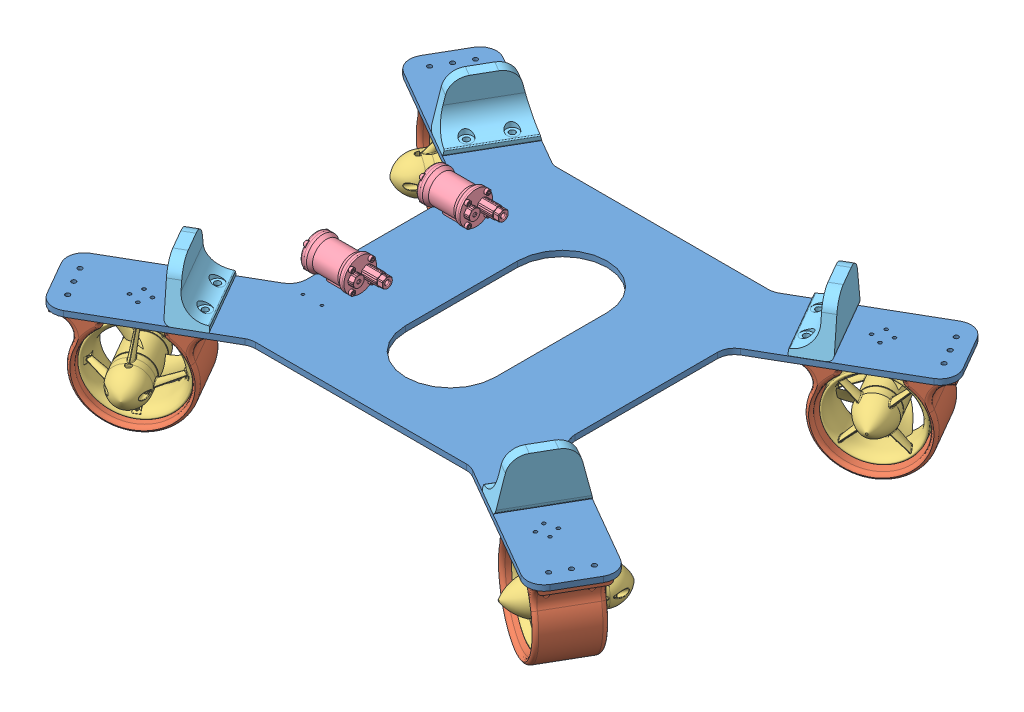
SolidWorks assembly CR-SA-003-HorizontalMotorsAndMount, configuration Default. Lengths in mm.
Overall size (620.81 551.29 537.72).
19 component instances, 5 part files, 40 mates.
Components (placement in the parent):
- CR-P-0008-MotorMount-1: CR-P-0008-MotorMount [Default] at (-219.9502 -31.4468 156.8428) x (0 0 -1) z (1 0 0) size (503.61 6.35 620.81)
- CR-SA-HorizontalThrusterAndMount-1: CR-SA-HorizontalThrusterAndMount [Default] at (-314.8315 -31.4468 365.9541) x (0.866025 0 -0.5) z (-0.5 0 -0.866025) size (139.7 110.81 112.68)
  - CR-P-0005b-Frame-MotorMount Horizontal-1: CR-P-0005b-Frame-MotorMount Horizontal [Default] at (0 55.5625 -5.427) x (0 -1 0) z (0 0 1) size (110.81 139.7 64.82)
  - CR-P-0003-T200-THRUSTER-R1-1: CR-P-0003-T200-THRUSTER-R1 [Default] at (0 55.5625 26.323) x (1 0 0) z (0 0 -1) size (96.71 97.53 112.68)
- CR-SA-HorizontalThrusterAndMount-2: CR-SA-HorizontalThrusterAndMount [Default] at (-341.1545 -31.4468 -6.6757) x (0.866025 0 0.5) z (0.5 0 -0.866025) size (139.7 110.81 112.68)
  - CR-P-0005b-Frame-MotorMount Horizontal-1: CR-P-0005b-Frame-MotorMount Horizontal [Default] at (0 55.5625 -5.427) x (0 -1 0) z (0 0 1) size (110.81 139.7 64.82)
  - CR-P-0003-T200-THRUSTER-R1-1: CR-P-0003-T200-THRUSTER-R1 [Default] at (0 55.5625 26.323) x (1 0 0) z (0 0 -1) size (96.71 97.53 112.68)
- CR-SA-HorizontalThrusterAndMount-3: CR-SA-HorizontalThrusterAndMount [Default] at (124.6163 -31.4468 -52.2686) x (-0.866025 0 0.5) z (0.5 0 0.866025) size (139.7 110.81 112.68)
  - CR-P-0005b-Frame-MotorMount Horizontal-1: CR-P-0005b-Frame-MotorMount Horizontal [Default] at (0 55.5625 -5.427) x (0 -1 0) z (0 0 1) size (110.81 139.7 64.82)
  - CR-P-0003-T200-THRUSTER-R1-1: CR-P-0003-T200-THRUSTER-R1 [Default] at (0 55.5625 26.323) x (1 0 0) z (0 0 -1) size (96.71 97.53 112.68)
- CR-SA-HorizontalThrusterAndMount-4: CR-SA-HorizontalThrusterAndMount [Default] at (150.9393 -31.4468 320.3613) x (-0.866025 0 -0.5) z (-0.5 0 0.866025) size (139.7 110.81 112.68)
  - CR-P-0005b-Frame-MotorMount Horizontal-1: CR-P-0005b-Frame-MotorMount Horizontal [Default] at (0 55.5625 -5.427) x (0 -1 0) z (0 0 1) size (110.81 139.7 64.82)
  - CR-P-0003-T200-THRUSTER-R1-1: CR-P-0003-T200-THRUSTER-R1 [Default] at (0 55.5625 26.323) x (1 0 0) z (0 0 -1) size (96.71 97.53 112.68)
- LUMEN-ASM-R3-PUBLIC-1: LUMEN-ASM-R3-PUBLIC [Default] at (-203.5576 -25.0968 -167.9027) x (0 1 0) z (1 0 0) size (38.48 37 78.39)
- LUMEN-ASM-R3-PUBLIC-4: LUMEN-ASM-R3-PUBLIC [Default] at (-203.5576 -25.0968 -299.4807) x (0 1 0) z (1 0 0) size (38.48 37 78.39)
- CR-P-RestingFeet-1: CR-P-RestingFeet [Default] at (-303.4208 3.4782 -15.1387) x (-0.5 0 0.866025) z (0 1 0) size (82.55 38.1 57.15)
- CR-P-RestingFeet-3: CR-P-RestingFeet [Default] at (113.0786 3.4782 -15.3587) x (-0.5 0 -0.866025) z (0 1 0) size (82.55 38.1 57.15)
- CR-P-RestingFeet-4: CR-P-RestingFeet [Default] at (-303.2938 3.4782 329.0442) x (0.5 0 0.866025) z (0 1 0) size (82.55 38.1 57.15)
- CR-P-RestingFeet-5: CR-P-RestingFeet [Default] at (113.2056 3.4782 328.8243) x (0.5 0 -0.866025) z (0 1 0) size (82.55 38.1 57.15)
Mates (geometry in assembly coordinates):
- Coincident2: coincident anti-aligned: plane of CR-P-0006-VectorizedMotorPlate-2 through (-82.6086 0 202.1216) normal (0 -1 0); plane of CR-P-0005b-Frame-MotorMount Horizontal-1 through (-332.933 -31.4468 4.4842) normal (0 1 0)
- Tangent1: tangent anti-aligned: plane of CR-P-0006-VectorizedMotorPlate-2 through (-312.1112 6.35 238.0427) normal (-0.707107 0 0.707107); cylinder of CR-P-0005b-Frame-MotorMount Horizontal-1 through (-389.1249 -26.674 398.9031) axis (0.707107 0 0.707107) radius 33.02
- Coincident6: coincident anti-aligned: plane of CR-P-0005b-Frame-MotorMount Horizontal-1 through (-332.933 -37.7968 4.4842) normal (0 -1 0); plane of CR-P-0003-T200-THRUSTER-R1-1 through (-372.3007 -37.7968 335.9963) normal (0 1 0)
- Coincident7: coincident anti-aligned: plane of CR-P-0006-VectorizedMotorPlate-2 through (-82.6086 0 202.1216) normal (0 -1 0); plane of CR-P-0005b-Frame-MotorMount Horizontal-2 through (-375.955 -31.4468 11.89) normal (0 1 0)
- Tangent3: tangent anti-aligned: plane of CR-P-0006-VectorizedMotorPlate-2 through (146.894 6.35 238.0427) normal (0.707107 0 0.707107); cylinder of CR-P-0005b-Frame-MotorMount Horizontal-2 through (-330.4009 -26.674 57.4441) axis (-0.707107 0 0.707107) radius 33.02
- Coincident9: coincident anti-aligned: plane of CR-P-0003-T200-THRUSTER-R1-2 through (-353.3308 -37.7968 -12.5208) normal (0 1 0); plane of CR-P-0005b-Frame-MotorMount Horizontal-2 through (-375.955 -37.7968 11.89) normal (0 -1 0)
- Coincident10: coincident anti-aligned: plane of CR-P-0005b-Frame-MotorMount Horizontal-2 through (-375.955 -31.4468 11.89) normal (0 1 0); plane of CR-P-0008-MotorMount-1 through (-219.9502 -31.4468 156.8428) normal (0 -1 0)
- Coincident13: coincident anti-aligned: plane of CR-P-0005b-Frame-MotorMount Horizontal-1 through (-332.933 -31.4468 4.4842) normal (0 1 0); plane of CR-P-0008-MotorMount-1 through (-219.9502 -31.4468 156.8428) normal (0 -1 0)
- Coincident14: coincident anti-aligned: plane of CR-P-0008-MotorMount-1 through (-219.9502 -31.4468 156.8428) normal (0 -1 0); plane of CR-SA-HorizontalThrusterAndMount-1/CR-P-0005b-Frame-MotorMount Horizontal-1 through (-343.868 -31.4468 315.6614) normal (0 1 0)
- Coincident15: coincident anti-aligned: plane of CR-P-0008-MotorMount-1 through (-219.9502 -31.4468 156.8428) normal (0 -1 0); plane of CR-SA-HorizontalThrusterAndMount-2/CR-P-0005b-Frame-MotorMount Horizontal-1 through (-312.118 -31.4468 -56.9684) normal (0 1 0)
- Angle1: planar angle = 2.094395 rad anti-aligned: plane of CR-SA-HorizontalThrusterAndMount-1/CR-P-0005b-Frame-MotorMount Horizontal-1 through (-343.868 -87.0093 315.6614) normal (-0.5 0 -0.866025); plane of CR-P-0008-MotorMount-1 through (-247.5076 -25.0968 248.8825) normal (-1 0 0)
- Angle2: planar angle = 2.094395 rad anti-aligned: plane of CR-P-0008-MotorMount-1 through (-247.5076 -25.0968 248.8825) normal (-1 0 0); plane of CR-SA-HorizontalThrusterAndMount-2/CR-P-0005b-Frame-MotorMount Horizontal-1 through (-343.868 -87.0093 -1.9758) normal (-0.5 0 0.866025)
- Coincident18: coincident anti-aligned: plane of CR-P-0008-MotorMount-1 through (-219.9502 -31.4468 156.8428) normal (0 -1 0); plane of CR-SA-HorizontalThrusterAndMount-3/CR-P-0005b-Frame-MotorMount Horizontal-1 through (153.6528 -31.4468 -1.9758) normal (0 1 0)
- Angle3: planar angle = 2.094395 rad anti-aligned: plane of CR-SA-HorizontalThrusterAndMount-3/CR-P-0005b-Frame-MotorMount Horizontal-1 through (153.6528 -87.0093 -1.9758) normal (0.5 0 0.866025); plane of CR-P-0008-MotorMount-1 through (57.2924 -25.0968 248.8825) normal (1 0 0)
- Coincident20: coincident anti-aligned: plane of CR-P-0008-MotorMount-1 through (-219.9502 -31.4468 156.8428) normal (0 -1 0); plane of CR-SA-HorizontalThrusterAndMount-4/CR-P-0005b-Frame-MotorMount Horizontal-1 through (121.9028 -31.4468 370.654) normal (0 1 0)
- Angle4: planar angle = 2.094395 rad anti-aligned: plane of CR-SA-HorizontalThrusterAndMount-4/CR-P-0005b-Frame-MotorMount Horizontal-1 through (153.6528 -87.0093 315.6614) normal (0.5 0 -0.866025); plane of CR-P-0008-MotorMount-1 through (57.2924 -25.0968 248.8825) normal (1 0 0)
- Coincident22: coincident anti-aligned: plane of CR-P-0008-MotorMount-1 through (-219.9502 -31.4468 156.8428) normal (0 -1 0); plane of CR-P-0005b-Frame-MotorMount Horizontal-1 through (-332.933 -31.4468 4.4842) normal (0 1 0)
- Distance2: distance = 3.81 mm aligned: plane of CR-P-0005b-Frame-MotorMount Horizontal-1 through (-393.4249 -87.0093 -30.4408) normal (-0.866025 0 -0.5); plane of CR-P-0008-MotorMount-1 through (-412.4854 -25.0968 -30.447) normal (-0.866025 0 -0.5)
- Distance3: distance = 9.525 mm aligned: plane of CR-P-0005b-Frame-MotorMount Horizontal-1 through (-301.183 -87.0093 -50.5085) normal (0.5 0 -0.866025); plane of CR-P-0008-MotorMount-1 through (-371.2104 -25.0968 -101.9373) normal (0.5 0 -0.866025)
- Coincident23: coincident anti-aligned: plane of CR-P-0008-MotorMount-1 through (-219.9502 -25.0968 156.8428) normal (0 1 0); plane of LUMEN-ASM-R3-PUBLIC-1 through (-203.5576 -25.0968 222.6318) normal (0 -1 0)
- Parallel1: parallel anti-aligned: line of CR-P-0008-MotorMount-1 through (-214.8458 -25.0968 328.2928) axis (1 0 0); cylinder of LUMEN-ASM-R3-PUBLIC-1 through (-203.5576 -5.1118 222.6318) axis (-1 0 0) radius 15.985
- Coincident25: coincident anti-aligned: plane of CR-P-0008-MotorMount-1 through (-219.9502 -25.0968 156.8428) normal (0 1 0); plane of LUMEN-ASM-R3-PUBLIC-3 through (-203.5576 -25.0968 205.6138) normal (0 -1 0)
- Concentric5: concentric anti-aligned: cylinder of CR-P-0008-MotorMount-1 through (-234.8076 -31.4468 222.6318) axis (0 1 0) radius 1.524; cylinder of LUMEN-ASM-R3-PUBLIC-3 through (-234.8076 -25.0968 205.6138) axis (0 -1 0) radius 1.25
- Parallel3: parallel aligned: cylinder of LUMEN-ASM-R3-PUBLIC-1 through (-203.5576 -5.1118 222.6318) axis (-1 0 0) radius 15.985; cylinder of LUMEN-ASM-R3-PUBLIC-3 through (-203.5576 -5.1118 205.6138) axis (-1 0 0) radius 15.985
- Coincident26: coincident anti-aligned: plane of CR-P-0008-MotorMount-1 through (-219.9502 -25.0968 156.8428) normal (0 1 0); plane of LUMEN-ASM-R3-PUBLIC-4 through (-203.5576 -25.0968 91.0538) normal (0 -1 0)
- Parallel5: parallel aligned: cylinder of LUMEN-ASM-R3-PUBLIC-3 through (-203.5576 -5.1118 205.6138) axis (-1 0 0) radius 15.985; cylinder of LUMEN-ASM-R3-PUBLIC-4 through (-203.5576 -5.1118 91.0538) axis (-1 0 0) radius 15.985
- Coincident32: coincident anti-aligned: plane of CR-P-0008-MotorMount-1 through (-219.9502 -25.0968 156.8428) normal (0 1 0); plane of CR-P-RestingFeet-2 through (-339.5528 -25.0968 357.5927) normal (0 -1 0)
- Coincident36: coincident aligned: line of CR-P-0008-MotorMount-1 through (-222.8973 -25.0968 -16.3087) axis (-0.866025 0 -0.5); line of CR-P-RestingFeet-1 through (-250.8875 -25.0968 -32.4689) axis (-0.866025 0 -0.5)
- Coincident37: coincident anti-aligned: line of CR-P-0008-MotorMount-1 through (-395.9877 -25.0968 -20.922) axis (0.866025 0 0.5); line of CR-P-RestingFeet-1 through (-292.1625 -25.0968 39.0215) axis (-0.866025 0 -0.5)
- Concentric9: concentric anti-aligned: cylinder of CR-P-0008-MotorMount-1 through (-234.8076 -31.4468 91.0538) axis (0 1 0) radius 1.524; cylinder of LUMEN-ASM-R3-PUBLIC-4 through (-234.8076 -25.0968 91.0538) axis (0 -1 0) radius 1.25
- Concentric10: concentric anti-aligned: circle of CR-P-0008-MotorMount-1; cylinder of LUMEN-ASM-R3-PUBLIC-1 through (-234.8076 -25.0968 222.6318) axis (0 -1 0) radius 1.25
- Coincident39: coincident anti-aligned: plane of CR-P-0008-MotorMount-1 through (-219.9502 -25.0968 156.8428) normal (0 1 0); plane of CR-P-RestingFeet-3 through (102.08 -25.0968 -9.0087) normal (0 -1 0)
- Concentric12: concentric aligned: circle of CR-P-0008-MotorMount-1; circle of CR-P-RestingFeet-3
- Concentric13: concentric aligned: circle of CR-P-0008-MotorMount-1; circle of CR-P-RestingFeet-3
- Coincident40: coincident anti-aligned: plane of CR-P-0008-MotorMount-1 through (-219.9502 -25.0968 156.8428) normal (0 1 0); plane of CR-P-RestingFeet-4 through (-292.2952 -25.0968 322.6942) normal (0 -1 0)
- Concentric14: concentric aligned: cylinder of CR-P-0008-MotorMount-1 through (-268.9747 -25.0968 331.0805) axis (0 -1 0) radius 2.54; cylinder of CR-P-RestingFeet-4 through (-268.9747 13.0032 331.0805) axis (0 -1 0) radius 3.429
- Concentric15: concentric aligned: cylinder of CR-P-0008-MotorMount-1 through (-288.0247 -25.0968 298.0849) axis (0 -1 0) radius 2.54; cylinder of CR-P-RestingFeet-4 through (-288.0247 13.0032 298.0849) axis (0 -1 0) radius 3.429
- Coincident43: coincident anti-aligned: plane of CR-P-0008-MotorMount-1 through (-219.9502 -25.0968 156.8428) normal (0 1 0); plane of CR-P-RestingFeet-5 through (102.207 -25.0968 322.4743) normal (0 -1 0)
- Concentric16: concentric aligned: cylinder of CR-P-0008-MotorMount-1 through (97.8095 -25.0968 298.0849) axis (0 -1 0) radius 2.54; cylinder of CR-P-RestingFeet-5 through (97.8095 13.0032 298.0849) axis (0 -1 0) radius 3.429
- Concentric17: concentric aligned: cylinder of CR-P-0008-MotorMount-1 through (78.7595 -25.0968 331.0805) axis (0 -1 0) radius 2.54; cylinder of CR-P-RestingFeet-5 through (78.7595 13.0032 331.0805) axis (0 -1 0) radius 3.429
